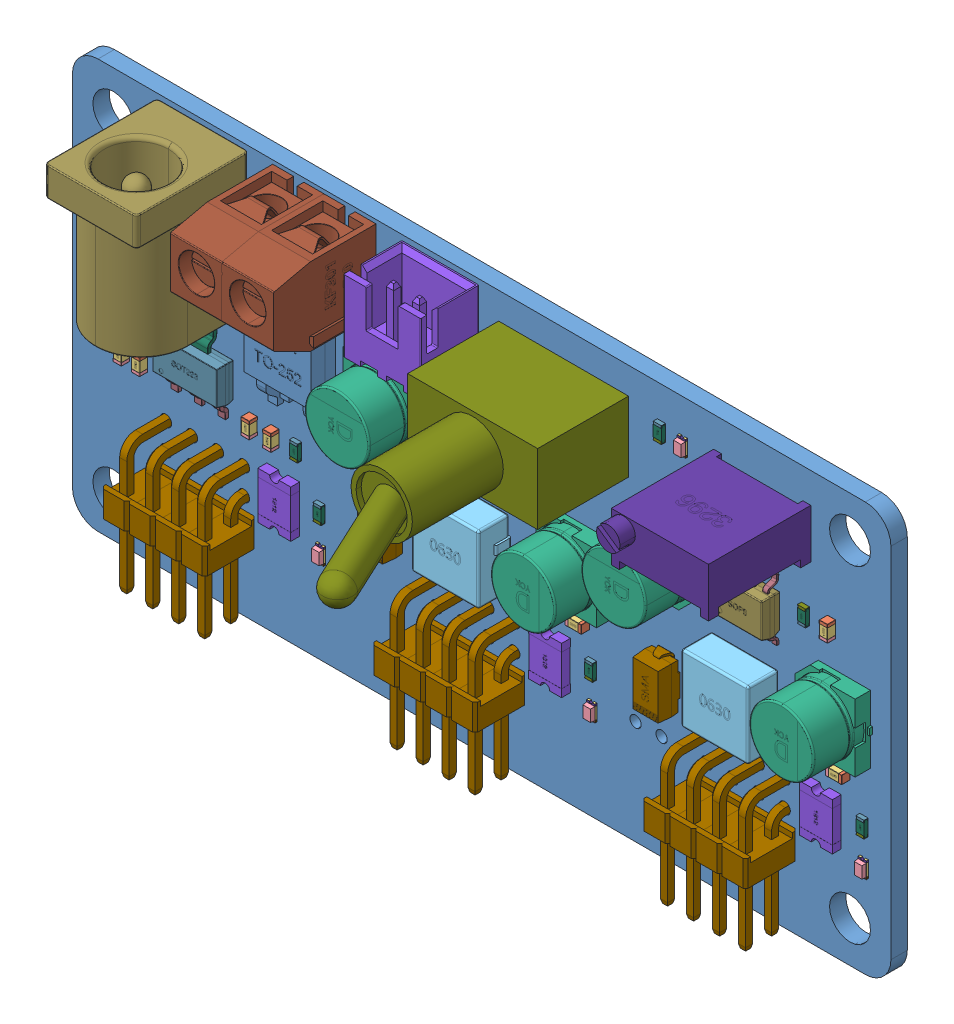
SolidWorks assembly PowerSupplyBoard, configuration 默认. Lengths in mm.
Overall size (80 40 32.5).
298 component instances, 37 part files, 0 mates.
Components (placement in the parent):
- PCB2.step-1: PCB2.step [默认] at origin size (80 40 32.5)
  - Board.step-1: Board.step [默认] at origin size (80 40 1.6)
    - Open CASCADE STEP translator 6.8 2.1.1.step-1: Open CASCADE STEP translator 6.8 2.1.1.step [默认] at (0 0 -1.6) size (80 40 1.6)
  - C1.step-1: C1.step [默认] at origin size (0.82 1.6 0.82)
    - C_0603.step-1: C_0603.step [默认] at (74.2189 27.7979 0.0254) x (0 -1 0) z (0 0 1) size (1.6 0.82 0.82)
      - C_0603-7177_AF0_ASM.step-1: C_0603-7177_AF0_ASM.step [默认] at origin size (1.6 0.82 0.82)
        - C_0603-683_AF0_ASM.step-1: C_0603-683_AF0_ASM.step [默认] at origin size (1.6 0.82 0.82)
          - 2_1_200.step-1: 2_1_200.step [默认] at origin size (0.3 0.82 0.82)
          - _1_1_20001.step-1: _1_1_20001.step [默认] at origin size (1 0.8 0.8)
          - 3_1_2_A.step-1: 3_1_2_A.step [默认] at origin size (0.3 0.82 0.82)
  - C3.step-1: C3.step [默认] at origin size (7 6.6 5.41)
    - CM_D(6.3X5.4).step-1: CM_D(6.3X5.4).step [默认] at (74.7014 21.0058 0) x (0 1 0) z (0 0 1) size (6.6 7 5.41)
      - LOGO_.step-1: LOGO_.step [默认] at (1.6383 0.2015 -0.0035) x (-1 0 0) z (0 0 -1) size (1.35 1.56 0.01)
      - CM_D(6.3X5.4)-0.step-1: CM_D(6.3X5.4)-0.step [默认] at origin size (6.6 7 5.41)
  - Open CASCADE STEP translator 6.8 2.4.step-1: Open CASCADE STEP translator 6.8 2.4.step [默认] at origin size (7.54 7.7 9.1)
    - XH2.54-2P_H.step-1: XH2.54-2P_H.step [默认] at (37.2618 32.1564 0.03) x (-1 0 0) z (0 1 0) size (7.54 9.1 7.7)
      - LOGO_-1.step-1: LOGO_-1.step [默认] at (-1.159 -0.003 2.4494) x (0 0 1) z (0 -1 0) size (0.9 1.04 0.01)
      - XH2.54-2P_H-2.step-1: XH2.54-2P_H-2.step [默认] at origin size (7.54 9.1 7.7)
  - Open CASCADE STEP translator 6.8 2.5.step-1: Open CASCADE STEP translator 6.8 2.5.step [默认] at origin size (10.16 12.85 8.1)
    - HDR-1x2_H.step-1: HDR-1x2_H.step [默认] at (40.6527 12.7 0) x (1 0 0) z (0 0 1) size (2.54 12.85 8.1)
      - HDR-1x2_H-3.step-1: HDR-1x2_H-3.step [默认] at origin size (2.54 12.85 8.1)
      - LOGO_-4.step-1: LOGO_-4.step [默认] at (0 -4.7829 0.017) x (-1 0 0) z (0 0 -1) size (0.9 1.04 0.01)
    - HDR-1x2_H.step-2: HDR-1x2_H.step [默认] at (43.1927 12.7 0) x (1 0 0) z (0 0 1) size (2.54 12.85 8.1)
      - HDR-1x2_H-3.step-1: HDR-1x2_H-3.step [默认] at origin size (2.54 12.85 8.1)
      - LOGO_-4.step-1: LOGO_-4.step [默认] at (0 -4.7829 0.017) x (-1 0 0) z (0 0 -1) size (0.9 1.04 0.01)
    - HDR-1x2_H.step-3: HDR-1x2_H.step [默认] at (35.5727 12.7 0) x (1 0 0) z (0 0 1) size (2.54 12.85 8.1)
      - HDR-1x2_H-3.step-1: HDR-1x2_H-3.step [默认] at origin size (2.54 12.85 8.1)
      - LOGO_-4.step-1: LOGO_-4.step [默认] at (0 -4.7829 0.017) x (-1 0 0) z (0 0 -1) size (0.9 1.04 0.01)
    - HDR-1x2_H.step-4: HDR-1x2_H.step [默认] at (38.1127 12.7 0) x (1 0 0) z (0 0 1) size (2.54 12.85 8.1)
      - HDR-1x2_H-3.step-1: HDR-1x2_H-3.step [默认] at origin size (2.54 12.85 8.1)
      - LOGO_-4.step-1: LOGO_-4.step [默认] at (0 -4.7829 0.017) x (-1 0 0) z (0 0 -1) size (0.9 1.04 0.01)
  - Open CASCADE STEP translator 6.8 2.6.step-1: Open CASCADE STEP translator 6.8 2.6.step [默认] at origin size (5 6.01 1.9)
    - SOP8.step-1: SOP8.step [默认] at (39.878 26.6954 0) x (0 1 0) z (0 0 1) size (6.01 5 1.9)
      - LOGO_0.25.step-1: LOGO_0.25.step [默认] at (0.0116 0 0.095) x (0 -1 0) z (0 0 -1) size (0.75 0.87 0.01)
      - SOP8_____.step-1: SOP8_____.step [默认] at origin size (3.6 5 1.8)
      - ____1.8_______.step-1: ____1.8_______.step [默认] at (1.8 1.91 1) x (0 1 0) z (0 0 1) size (0.5 1.2 1.1)
      - ____1.8_______.step-2: ____1.8_______.step [默认] at (1.8 0.64 1) x (0 1 0) z (0 0 1) size (0.5 1.2 1.1)
      - ____1.8_______.step-3: ____1.8_______.step [默认] at (1.8 -0.63 1) x (0 1 0) z (0 0 1) size (0.5 1.2 1.1)
      - ____1.8_______.step-4: ____1.8_______.step [默认] at (1.8 -1.9 1) x (0 1 0) z (0 0 1) size (0.5 1.2 1.1)
      - ____1.8_______.step-5: ____1.8_______.step [默认] at (-1.8 1.91 1) x (0 -1 0) z (0 0 1) size (0.5 1.2 1.1)
      - ____1.8_______.step-6: ____1.8_______.step [默认] at (-1.8 0.64 1) x (0 -1 0) z (0 0 1) size (0.5 1.2 1.1)
      - ____1.8_______.step-7: ____1.8_______.step [默认] at (-1.8 -0.63 1) x (0 -1 0) z (0 0 1) size (0.5 1.2 1.1)
      - ____1.8_______.step-8: ____1.8_______.step [默认] at (-1.8 -1.9 1) x (0 -1 0) z (0 0 1) size (0.5 1.2 1.1)
  - Open CASCADE STEP translator 6.8 2.7.step-1: Open CASCADE STEP translator 6.8 2.7.step [默认] at origin size (5 6.01 1.9)
    - SOP8.step-1: SOP8.step [默认] at (66.9036 26.6954 0) x (0 1 0) z (0 0 1) size (6.01 5 1.9)
      - LOGO_0.25.step-1: LOGO_0.25.step [默认] at (0.0116 0 0.095) x (0 -1 0) z (0 0 -1) size (0.75 0.87 0.01)
      - SOP8_____.step-1: SOP8_____.step [默认] at origin size (3.6 5 1.8)
      - ____1.8_______.step-1: ____1.8_______.step [默认] at (1.8 1.91 1) x (0 1 0) z (0 0 1) size (0.5 1.2 1.1)
      - ____1.8_______.step-2: ____1.8_______.step [默认] at (1.8 0.64 1) x (0 1 0) z (0 0 1) size (0.5 1.2 1.1)
      - ____1.8_______.step-3: ____1.8_______.step [默认] at (1.8 -0.63 1) x (0 1 0) z (0 0 1) size (0.5 1.2 1.1)
      - ____1.8_______.step-4: ____1.8_______.step [默认] at (1.8 -1.9 1) x (0 1 0) z (0 0 1) size (0.5 1.2 1.1)
      - ____1.8_______.step-5: ____1.8_______.step [默认] at (-1.8 1.91 1) x (0 -1 0) z (0 0 1) size (0.5 1.2 1.1)
      - ____1.8_______.step-6: ____1.8_______.step [默认] at (-1.8 0.64 1) x (0 -1 0) z (0 0 1) size (0.5 1.2 1.1)
      - ____1.8_______.step-7: ____1.8_______.step [默认] at (-1.8 -0.63 1) x (0 -1 0) z (0 0 1) size (0.5 1.2 1.1)
      - ____1.8_______.step-8: ____1.8_______.step [默认] at (-1.8 -1.9 1) x (0 -1 0) z (0 0 1) size (0.5 1.2 1.1)
  - R6.step-1: R6.step [默认] at origin size (0.8 1.6 0.4)
    - R0603.step-1: R0603.step [默认] at (44.6277 27.5996 0) x (0 1 0) z (0 0 1) size (1.6 0.8 0.4)
      - R_0603-3615_AF0_ASM.step-1: R_0603-3615_AF0_ASM.step [默认] at origin size (1.6 0.8 0.4)
        - R_0603-3601_AF0_ASM.step-1: R_0603-3601_AF0_ASM.step [默认] at origin size (1.6 0.8 0.4)
          - _2_1_2_3_4_AF0.step-1: _2_1_2_3_4_AF0.step [默认] at origin size (0.25 0.8 0.4)
          - _7_1_2_AF0.step-1: _7_1_2_AF0.step [默认] at origin size (1.5 0.8 0.4)
          - 5_1_2_3_400.step-1: 5_1_2_3_400.step [默认] at origin size (0.25 0.8 0.4)
  - R5.step-1: R5.step [默认] at origin size (0.8 1.6 0.4)
    - R0603.step-1: R0603.step [默认] at (50.8338 12.5832 0) x (0 -1 0) z (0 0 1) size (1.6 0.8 0.4)
      - R_0603-3615_AF0_ASM.step-1: R_0603-3615_AF0_ASM.step [默认] at origin size (1.6 0.8 0.4)
        - R_0603-3601_AF0_ASM.step-1: R_0603-3601_AF0_ASM.step [默认] at origin size (1.6 0.8 0.4)
          - _2_1_2_3_4_AF0.step-1: _2_1_2_3_4_AF0.step [默认] at origin size (0.25 0.8 0.4)
          - _7_1_2_AF0.step-1: _7_1_2_AF0.step [默认] at origin size (1.5 0.8 0.4)
          - 5_1_2_3_400.step-1: 5_1_2_3_400.step [默认] at origin size (0.25 0.8 0.4)
  - R4.step-1: R4.step [默认] at origin size (0.8 1.6 0.4)
    - R0603.step-1: R0603.step [默认] at (47.2185 27.5996 0) x (0 1 0) z (0 0 1) size (1.6 0.8 0.4)
      - R_0603-3615_AF0_ASM.step-1: R_0603-3615_AF0_ASM.step [默认] at origin size (1.6 0.8 0.4)
        - R_0603-3601_AF0_ASM.step-1: R_0603-3601_AF0_ASM.step [默认] at origin size (1.6 0.8 0.4)
          - _2_1_2_3_4_AF0.step-1: _2_1_2_3_4_AF0.step [默认] at origin size (0.25 0.8 0.4)
          - _7_1_2_AF0.step-1: _7_1_2_AF0.step [默认] at origin size (1.5 0.8 0.4)
          - 5_1_2_3_400.step-1: 5_1_2_3_400.step [默认] at origin size (0.25 0.8 0.4)
  - LED2.step-1: LED2.step [默认] at origin size (0.8 1.6 0.61)
    - LED_0603-G(1).step-1: LED_0603-G(1).step [默认] at (50.8649 9.0649 0) x (0 1 0) z (0 0 1) size (1.6 0.8 0.47)
      - LED_0603-G-7058_AF0_ASM.step-1: LED_0603-G-7058_AF0_ASM.step [默认] at origin size (1.6 0.8 0.47)
        - LED_0603-G-4339_AF0_ASM.step-1: LED_0603-G-4339_AF0_ASM.step [默认] at origin size (1.6 0.8 0.47)
          - 4_100.step-1: 4_100.step [默认] at origin size (0.2 0.8 0.2)
          - _2_10001.step-1: _2_10001.step [默认] at origin size (0.2 0.8 0.2)
          - _5_2__10001.step-1: _5_2__10001.step [默认] at origin size (0.31 0.14 0)
          - _5_1__10001.step-1: _5_1__10001.step [默认] at origin size (0.31 0.14 0)
          - 1_1_2_3_4_5_6_7_8_0.step-1: 1_1_2_3_4_5_6_7_8_0.step [默认] at origin size (1.6 0.8 0.47)
    - LED_0603______.step-1: LED_0603______.step [默认] at (50.8649 9.0649 0) x (0 -1 0) z (0 0 1) size (1.2 0.8 0.4)
  - Open CASCADE STEP translator 6.8 2.12.step-1: Open CASCADE STEP translator 6.8 2.12.step [默认] at origin size (6.95 6.6 3.03)
    - SMD-0630.step-1: SMD-0630.step [默认] at (39.4682 18.3134 0) x (1 0 0) z (0 0 1) size (6.95 6.6 3.03)
      - SMD-0630-5.step-1: SMD-0630-5.step [默认] at origin size (6.95 6.6 3.03)
      - LOGO_0.5.step-1: LOGO_0.5.step [默认] at (0 0.0017 0.04) size (1.5 1.73 0.01)
  - F2.step-1: F2.step [默认] at origin size (3.22 4.6 0.87)
    - FU_01812.step-1: FU_01812.step [默认] at (47.0662 11.7496 0) x (0 -1 0) z (0 0 1) size (4.6 3.22 0.87)
      - LOGO_-6.step-1: LOGO_-6.step [默认] at (0 0.0363 0.009) x (-1 0 0) z (0 0 -1) size (0.6 0.69 0)
      - FU_1812.step-1: FU_1812.step [默认] at origin size (4.6 3.22 0.87)
  - D2.step-1: D2.step [默认] at origin size (2.6 5.12 2.1)
    - SMA.step-1: SMA.step [默认] at (31.2327 15.471 0.0508) x (0 1 0) z (0 0 1) size (5.12 2.6 2.1)
      - SMA-4715_AF0_ASM.step-1: SMA-4715_AF0_ASM.step [默认] at origin size (5.12 2.6 2.1)
        - SMA-5401_AF0.step-1: SMA-5401_AF0.step [默认] at origin size (5.12 2.6 2.1)
  - C12.step-1: C12.step [默认] at origin size (0.82 1.6 0.82)
    - C_0603.step-1: C_0603.step [默认] at (6.9851 16.7489 0.0254) x (0 -1 0) z (0 0 1) size (1.6 0.82 0.82)
      - C_0603-7177_AF0_ASM.step-1: C_0603-7177_AF0_ASM.step [默认] at origin size (1.6 0.82 0.82)
        - C_0603-683_AF0_ASM.step-1: C_0603-683_AF0_ASM.step [默认] at origin size (1.6 0.82 0.82)
          - 2_1_200.step-1: 2_1_200.step [默认] at origin size (0.3 0.82 0.82)
          - _1_1_20001.step-1: _1_1_20001.step [默认] at origin size (1 0.8 0.8)
          - 3_1_2_A.step-1: 3_1_2_A.step [默认] at origin size (0.3 0.82 0.82)
  - C10.step-1: C10.step [默认] at origin size (0.82 1.6 0.82)
    - C_0603.step-1: C_0603.step [默认] at (19.8248 16.7489 0.0254) x (0 -1 0) z (0 0 1) size (1.6 0.82 0.82)
      - C_0603-7177_AF0_ASM.step-1: C_0603-7177_AF0_ASM.step [默认] at origin size (1.6 0.82 0.82)
        - C_0603-683_AF0_ASM.step-1: C_0603-683_AF0_ASM.step [默认] at origin size (1.6 0.82 0.82)
          - 2_1_200.step-1: 2_1_200.step [默认] at origin size (0.3 0.82 0.82)
          - _1_1_20001.step-1: _1_1_20001.step [默认] at origin size (1 0.8 0.8)
          - 3_1_2_A.step-1: 3_1_2_A.step [默认] at origin size (0.3 0.82 0.82)
  - C9.step-1: C9.step [默认] at origin size (1.6 0.82 0.82)
    - C_0603.step-1: C_0603.step [默认] at (49.7689 16.1289 0.0254) x (-1 0 0) z (0 0 1) size (1.6 0.82 0.82)
      - C_0603-7177_AF0_ASM.step-1: C_0603-7177_AF0_ASM.step [默认] at origin size (1.6 0.82 0.82)
        - C_0603-683_AF0_ASM.step-1: C_0603-683_AF0_ASM.step [默认] at origin size (1.6 0.82 0.82)
          - 2_1_200.step-1: 2_1_200.step [默认] at origin size (0.3 0.82 0.82)
          - _1_1_20001.step-1: _1_1_20001.step [默认] at origin size (1 0.8 0.8)
          - 3_1_2_A.step-1: 3_1_2_A.step [默认] at origin size (0.3 0.82 0.82)
  - C8.step-1: C8.step [默认] at origin size (0.82 1.6 0.82)
    - C_0603.step-1: C_0603.step [默认] at (35.9681 25.8961 0.0254) x (0 -1 0) z (0 0 1) size (1.6 0.82 0.82)
      - C_0603-7177_AF0_ASM.step-1: C_0603-7177_AF0_ASM.step [默认] at origin size (1.6 0.82 0.82)
        - C_0603-683_AF0_ASM.step-1: C_0603-683_AF0_ASM.step [默认] at origin size (1.6 0.82 0.82)
          - 2_1_200.step-1: 2_1_200.step [默认] at origin size (0.3 0.82 0.82)
          - _1_1_20001.step-1: _1_1_20001.step [默认] at origin size (1 0.8 0.8)
          - 3_1_2_A.step-1: 3_1_2_A.step [默认] at origin size (0.3 0.82 0.82)
  - C7.step-1: C7.step [默认] at origin size (7 6.6 5.41)
    - CM_D(6.3X5.4).step-1: CM_D(6.3X5.4).step [默认] at (49.4284 21.0058 0) x (0 1 0) z (0 0 1) size (6.6 7 5.41)
      - LOGO_.step-1: LOGO_.step [默认] at (1.6383 0.2015 -0.0035) x (-1 0 0) z (0 0 -1) size (1.35 1.56 0.01)
      - CM_D(6.3X5.4)-0.step-1: CM_D(6.3X5.4)-0.step [默认] at origin size (6.6 7 5.41)
  - C6.step-1: C6.step [默认] at origin size (6.6 7 5.41)
    - CM_D(6.3X5.4).step-1: CM_D(6.3X5.4).step [默认] at (31.242 25.8318 0) x (-1 0 0) z (0 0 1) size (6.6 7 5.41)
      - LOGO_.step-1: LOGO_.step [默认] at (1.6383 0.2015 -0.0035) x (-1 0 0) z (0 0 -1) size (1.35 1.56 0.01)
      - CM_D(6.3X5.4)-0.step-1: CM_D(6.3X5.4)-0.step [默认] at origin size (6.6 7 5.41)
  - C13.step-1: C13.step [默认] at origin size (0.82 1.6 0.82)
    - C_0603.step-1: C_0603.step [默认] at (5.2071 16.7489 0.0254) x (0 -1 0) z (0 0 1) size (1.6 0.82 0.82)
      - C_0603-7177_AF0_ASM.step-1: C_0603-7177_AF0_ASM.step [默认] at origin size (1.6 0.82 0.82)
        - C_0603-683_AF0_ASM.step-1: C_0603-683_AF0_ASM.step [默认] at origin size (1.6 0.82 0.82)
          - 2_1_200.step-1: 2_1_200.step [默认] at origin size (0.3 0.82 0.82)
          - _1_1_20001.step-1: _1_1_20001.step [默认] at origin size (1 0.8 0.8)
          - 3_1_2_A.step-1: 3_1_2_A.step [默认] at origin size (0.3 0.82 0.82)
  - Open CASCADE STEP translator 6.8 2.22.step-1: Open CASCADE STEP translator 6.8 2.22.step [默认] at origin size (10.5 7.6 13.8)
    - KF301.step-1: KF301.step [默认] at (27.1742 36.6776 0.05) x (-1 0 0) z (0 0 1) size (5.5 7.6 13.8)
      - LOGO_-7.step-1: LOGO_-7.step [默认] at (0 1.4435 -0.0028) x (-1 0 0) z (0 0 -1) size (0.84 0.97 0.01)
      - KF301-8.step-1: KF301-8.step [默认] x (1 0 0) z (0 -1 0) size (5.5 13.8 7.6)
    - KF301.step-2: KF301.step [默认] at (22.1742 36.6776 0.05) x (-1 0 0) z (0 0 1) size (5.5 7.6 13.8)
      - LOGO_-7.step-1: LOGO_-7.step [默认] at (0 1.4435 -0.0028) x (-1 0 0) z (0 0 -1) size (0.84 0.97 0.01)
      - KF301-8.step-1: KF301-8.step [默认] x (1 0 0) z (0 -1 0) size (5.5 13.8 7.6)
  - Open CASCADE STEP translator 6.8 2.23.step-1: Open CASCADE STEP translator 6.8 2.23.step [默认] at origin size (9.3 14.05 15)
    - dc-005.step-1: dc-005.step [默认] at (12.9532 32.2582 0.2) x (-1 0 0) z (0 0 1) size (9.3 14.05 15)
  - C5.step-1: C5.step [默认] at origin size (1.6 0.82 0.82)
    - C_0603.step-1: C_0603.step [默认] at (75.2197 16.1289 0.0254) x (-1 0 0) z (0 0 1) size (1.6 0.82 0.82)
      - C_0603-7177_AF0_ASM.step-1: C_0603-7177_AF0_ASM.step [默认] at origin size (1.6 0.82 0.82)
        - C_0603-683_AF0_ASM.step-1: C_0603-683_AF0_ASM.step [默认] at origin size (1.6 0.82 0.82)
          - 2_1_200.step-1: 2_1_200.step [默认] at origin size (0.3 0.82 0.82)
          - _1_1_20001.step-1: _1_1_20001.step [默认] at origin size (1 0.8 0.8)
          - 3_1_2_A.step-1: 3_1_2_A.step [默认] at origin size (0.3 0.82 0.82)
  - Open CASCADE STEP translator 6.8 2.25.step-1: Open CASCADE STEP translator 6.8 2.25.step [默认] at origin size (6.51 7.02 1.67)
    - SOT223.step-1: SOT223.step [默认] at (12.6231 19.5037 0) x (1 0 0) z (0 0 1) size (6.51 7.02 1.67)
      - SOT223-4091_AF0_ASM.step-1: SOT223-4091_AF0_ASM.step [默认] at origin size (6.51 7.02 1.67)
        - SOT223_-20.step-1: SOT223_-20.step [默认] at (-2.3 -1.75 0.725) x (-1 0 0) z (0 0 1) size (0.71 1.76 0.92)
        - SOT223-16115_AF0.step-1: SOT223-16115_AF0.step [默认] at origin size (6.51 3.51 1.6)
        - SOT223_-10.step-1: SOT223_-10.step [默认] at (0 1.75 0.725) size (3 1.76 0.92)
        - SOT223_-20.step-2: SOT223_-20.step [默认] at (2.3 -1.75 0.725) x (-1 0 0) z (0 0 1) size (0.71 1.76 0.92)
        - SOT223_-20.step-3: SOT223_-20.step [默认] at (0 -1.75 0.725) x (-1 0 0) z (0 0 1) size (0.71 1.76 0.92)
  - S1.step-1: S1.step [默认] at origin size (12.72 10.16 32.39)
    - User_Library-7101SYZQE_switch-toggle.step-1: User_Library-7101SYZQE_switch-toggle.step [默认] at (48.26 34.2138 9.144) x (0 0 -1) z (1 0 0) size (32.39 10.16 12.72)
  - R9.step-1: R9.step [默认] at origin size (0.8 1.6 0.4)
    - R0603.step-1: R0603.step [默认] at (57.5666 36.0794 0) x (0 -1 0) z (0 0 1) size (1.6 0.8 0.4)
      - R_0603-3615_AF0_ASM.step-1: R_0603-3615_AF0_ASM.step [默认] at origin size (1.6 0.8 0.4)
        - R_0603-3601_AF0_ASM.step-1: R_0603-3601_AF0_ASM.step [默认] at origin size (1.6 0.8 0.4)
          - _2_1_2_3_4_AF0.step-1: _2_1_2_3_4_AF0.step [默认] at origin size (0.25 0.8 0.4)
          - _7_1_2_AF0.step-1: _7_1_2_AF0.step [默认] at origin size (1.5 0.8 0.4)
          - 5_1_2_3_400.step-1: 5_1_2_3_400.step [默认] at origin size (0.25 0.8 0.4)
  - R8.step-1: R8.step [默认] at origin size (0.8 1.6 0.4)
    - R0603.step-1: R0603.step [默认] at (21.9965 16.7234 0) x (0 -1 0) z (0 0 1) size (1.6 0.8 0.4)
      - R_0603-3615_AF0_ASM.step-1: R_0603-3615_AF0_ASM.step [默认] at origin size (1.6 0.8 0.4)
        - R_0603-3601_AF0_ASM.step-1: R_0603-3601_AF0_ASM.step [默认] at origin size (1.6 0.8 0.4)
          - _2_1_2_3_4_AF0.step-1: _2_1_2_3_4_AF0.step [默认] at origin size (0.25 0.8 0.4)
          - _7_1_2_AF0.step-1: _7_1_2_AF0.step [默认] at origin size (1.5 0.8 0.4)
          - 5_1_2_3_400.step-1: 5_1_2_3_400.step [默认] at origin size (0.25 0.8 0.4)
  - R7.step-1: R7.step [默认] at origin size (0.8 1.6 0.4)
    - R0603.step-1: R0603.step [默认] at (24.2991 12.5832 0) x (0 -1 0) z (0 0 1) size (1.6 0.8 0.4)
      - R_0603-3615_AF0_ASM.step-1: R_0603-3615_AF0_ASM.step [默认] at origin size (1.6 0.8 0.4)
        - R_0603-3601_AF0_ASM.step-1: R_0603-3601_AF0_ASM.step [默认] at origin size (1.6 0.8 0.4)
          - _2_1_2_3_4_AF0.step-1: _2_1_2_3_4_AF0.step [默认] at origin size (0.25 0.8 0.4)
          - _7_1_2_AF0.step-1: _7_1_2_AF0.step [默认] at origin size (1.5 0.8 0.4)
          - 5_1_2_3_400.step-1: 5_1_2_3_400.step [默认] at origin size (0.25 0.8 0.4)
  - R3.step-1: R3.step [默认] at origin size (0.8 1.6 0.4)
    - R0603.step-1: R0603.step [默认] at (77.3685 12.5832 0) x (0 -1 0) z (0 0 1) size (1.6 0.8 0.4)
      - R_0603-3615_AF0_ASM.step-1: R_0603-3615_AF0_ASM.step [默认] at origin size (1.6 0.8 0.4)
        - R_0603-3601_AF0_ASM.step-1: R_0603-3601_AF0_ASM.step [默认] at origin size (1.6 0.8 0.4)
          - _2_1_2_3_4_AF0.step-1: _2_1_2_3_4_AF0.step [默认] at origin size (0.25 0.8 0.4)
          - _7_1_2_AF0.step-1: _7_1_2_AF0.step [默认] at origin size (1.5 0.8 0.4)
          - 5_1_2_3_400.step-1: 5_1_2_3_400.step [默认] at origin size (0.25 0.8 0.4)
  - R2.step-1: R2.step [默认] at origin size (9.5 4.8 15)
    - 3296.step-1: 3296.step [默认] at (67.4409 34.6711 0.02) x (-1 0 0) z (0 0 1) size (9.5 4.8 15)
      - 3296-10.step-1: 3296-10.step [默认] at origin size (9.5 4.8 15)
      - LOGO_-11.step-1: LOGO_-11.step [默认] at (1.2121 -0.8676 0.494) x (-1 0 0) z (0 0 -1) size (1.8 2.08 0.01)
  - R1.step-1: R1.step [默认] at origin size (0.8 1.6 0.4)
    - R0603.step-1: R0603.step [默认] at (71.6533 27.5996 0) x (0 1 0) z (0 0 1) size (1.6 0.8 0.4)
      - R_0603-3615_AF0_ASM.step-1: R_0603-3615_AF0_ASM.step [默认] at origin size (1.6 0.8 0.4)
        - R_0603-3601_AF0_ASM.step-1: R_0603-3601_AF0_ASM.step [默认] at origin size (1.6 0.8 0.4)
          - _2_1_2_3_4_AF0.step-1: _2_1_2_3_4_AF0.step [默认] at origin size (0.25 0.8 0.4)
          - _7_1_2_AF0.step-1: _7_1_2_AF0.step [默认] at origin size (1.5 0.8 0.4)
          - 5_1_2_3_400.step-1: 5_1_2_3_400.step [默认] at origin size (0.25 0.8 0.4)
  - Q1.step-1: Q1.step [默认] at origin size (6.73 10.1 2.4)
    - DPAK_TO-252AA.step-1: DPAK_TO-252AA.step [默认] at (22.5553 26.1736 0.127) x (1 0 0) z (0 -1 0) size (6.73 2.4 10.1)
  - LED4.step-1: LED4.step [默认] at origin size (0.8 1.6 0.61)
    - LED_0603-G(1).step-1: LED_0603-G(1).step [默认] at (59.7183 35.8962 0) x (0 1 0) z (0 0 1) size (1.6 0.8 0.47)
      - LED_0603-G-7058_AF0_ASM.step-1: LED_0603-G-7058_AF0_ASM.step [默认] at origin size (1.6 0.8 0.47)
        - LED_0603-G-4339_AF0_ASM.step-1: LED_0603-G-4339_AF0_ASM.step [默认] at origin size (1.6 0.8 0.47)
          - 4_100.step-1: 4_100.step [默认] at origin size (0.2 0.8 0.2)
          - _2_10001.step-1: _2_10001.step [默认] at origin size (0.2 0.8 0.2)
          - _5_2__10001.step-1: _5_2__10001.step [默认] at origin size (0.31 0.14 0)
          - _5_1__10001.step-1: _5_1__10001.step [默认] at origin size (0.31 0.14 0)
          - 1_1_2_3_4_5_6_7_8_0.step-1: 1_1_2_3_4_5_6_7_8_0.step [默认] at origin size (1.6 0.8 0.47)
    - LED_0603______.step-1: LED_0603______.step [默认] at (59.7183 35.8962 0) x (0 -1 0) z (0 0 1) size (1.2 0.8 0.4)
  - LED3.step-1: LED3.step [默认] at origin size (0.8 1.6 0.61)
    - LED_0603-G(1).step-1: LED_0603-G(1).step [默认] at (24.3395 9.0649 0) x (0 1 0) z (0 0 1) size (1.6 0.8 0.47)
      - LED_0603-G-7058_AF0_ASM.step-1: LED_0603-G-7058_AF0_ASM.step [默认] at origin size (1.6 0.8 0.47)
        - LED_0603-G-4339_AF0_ASM.step-1: LED_0603-G-4339_AF0_ASM.step [默认] at origin size (1.6 0.8 0.47)
          - 4_100.step-1: 4_100.step [默认] at origin size (0.2 0.8 0.2)
          - _2_10001.step-1: _2_10001.step [默认] at origin size (0.2 0.8 0.2)
          - _5_2__10001.step-1: _5_2__10001.step [默认] at origin size (0.31 0.14 0)
          - _5_1__10001.step-1: _5_1__10001.step [默认] at origin size (0.31 0.14 0)
          - 1_1_2_3_4_5_6_7_8_0.step-1: 1_1_2_3_4_5_6_7_8_0.step [默认] at origin size (1.6 0.8 0.47)
    - LED_0603______.step-1: LED_0603______.step [默认] at (24.3395 9.0649 0) x (0 -1 0) z (0 0 1) size (1.2 0.8 0.4)
  - LED1.step-1: LED1.step [默认] at origin size (0.8 1.6 0.61)
    - LED_0603-G(1).step-1: LED_0603-G(1).step [默认] at (77.3902 9.0649 0) x (0 1 0) z (0 0 1) size (1.6 0.8 0.47)
      - LED_0603-G-7058_AF0_ASM.step-1: LED_0603-G-7058_AF0_ASM.step [默认] at origin size (1.6 0.8 0.47)
        - LED_0603-G-4339_AF0_ASM.step-1: LED_0603-G-4339_AF0_ASM.step [默认] at origin size (1.6 0.8 0.47)
          - 4_100.step-1: 4_100.step [默认] at origin size (0.2 0.8 0.2)
          - _2_10001.step-1: _2_10001.step [默认] at origin size (0.2 0.8 0.2)
          - _5_2__10001.step-1: _5_2__10001.step [默认] at origin size (0.31 0.14 0)
          - _5_1__10001.step-1: _5_1__10001.step [默认] at origin size (0.31 0.14 0)
          - 1_1_2_3_4_5_6_7_8_0.step-1: 1_1_2_3_4_5_6_7_8_0.step [默认] at origin size (1.6 0.8 0.47)
    - LED_0603______.step-1: LED_0603______.step [默认] at (77.3902 9.0649 0) x (0 -1 0) z (0 0 1) size (1.2 0.8 0.4)
  - Open CASCADE STEP translator 6.8 2.37.step-1: Open CASCADE STEP translator 6.8 2.37.step [默认] at origin size (6.95 6.6 3.03)
    - SMD-0630.step-1: SMD-0630.step [默认] at (65.808 18.3134 0) x (1 0 0) z (0 0 1) size (6.95 6.6 3.03)
      - SMD-0630-5.step-1: SMD-0630-5.step [默认] at origin size (6.95 6.6 3.03)
      - LOGO_0.5.step-1: LOGO_0.5.step [默认] at (0 0.0017 0.04) size (1.5 1.73 0.01)
  - Open CASCADE STEP translator 6.8 2.38.step-1: Open CASCADE STEP translator 6.8 2.38.step [默认] at origin size (10.16 12.85 8.1)
    - HDR-1x2_H.step-1: HDR-1x2_H.step [默认] at (14.224 12.7 0) x (1 0 0) z (0 0 1) size (2.54 12.85 8.1)
      - HDR-1x2_H-3.step-1: HDR-1x2_H-3.step [默认] at origin size (2.54 12.85 8.1)
      - LOGO_-4.step-1: LOGO_-4.step [默认] at (0 -4.7829 0.017) x (-1 0 0) z (0 0 -1) size (0.9 1.04 0.01)
    - HDR-1x2_H.step-2: HDR-1x2_H.step [默认] at (16.764 12.7 0) x (1 0 0) z (0 0 1) size (2.54 12.85 8.1)
      - HDR-1x2_H-3.step-1: HDR-1x2_H-3.step [默认] at origin size (2.54 12.85 8.1)
      - LOGO_-4.step-1: LOGO_-4.step [默认] at (0 -4.7829 0.017) x (-1 0 0) z (0 0 -1) size (0.9 1.04 0.01)
    - HDR-1x2_H.step-3: HDR-1x2_H.step [默认] at (9.144 12.7 0) x (1 0 0) z (0 0 1) size (2.54 12.85 8.1)
      - HDR-1x2_H-3.step-1: HDR-1x2_H-3.step [默认] at origin size (2.54 12.85 8.1)
      - LOGO_-4.step-1: LOGO_-4.step [默认] at (0 -4.7829 0.017) x (-1 0 0) z (0 0 -1) size (0.9 1.04 0.01)
    - HDR-1x2_H.step-4: HDR-1x2_H.step [默认] at (11.684 12.7 0) x (1 0 0) z (0 0 1) size (2.54 12.85 8.1)
      - HDR-1x2_H-3.step-1: HDR-1x2_H-3.step [默认] at origin size (2.54 12.85 8.1)
      - LOGO_-4.step-1: LOGO_-4.step [默认] at (0 -4.7829 0.017) x (-1 0 0) z (0 0 -1) size (0.9 1.04 0.01)
  - Open CASCADE STEP translator 6.8 2.39.step-1: Open CASCADE STEP translator 6.8 2.39.step [默认] at origin size (10.16 12.85 8.1)
    - HDR-1x2_H.step-1: HDR-1x2_H.step [默认] at (67.0814 12.7 0) x (1 0 0) z (0 0 1) size (2.54 12.85 8.1)
      - HDR-1x2_H-3.step-1: HDR-1x2_H-3.step [默认] at origin size (2.54 12.85 8.1)
      - LOGO_-4.step-1: LOGO_-4.step [默认] at (0 -4.7829 0.017) x (-1 0 0) z (0 0 -1) size (0.9 1.04 0.01)
    - HDR-1x2_H.step-2: HDR-1x2_H.step [默认] at (69.6214 12.7 0) x (1 0 0) z (0 0 1) size (2.54 12.85 8.1)
      - HDR-1x2_H-3.step-1: HDR-1x2_H-3.step [默认] at origin size (2.54 12.85 8.1)
      - LOGO_-4.step-1: LOGO_-4.step [默认] at (0 -4.7829 0.017) x (-1 0 0) z (0 0 -1) size (0.9 1.04 0.01)
    - HDR-1x2_H.step-3: HDR-1x2_H.step [默认] at (62.0014 12.7 0) x (1 0 0) z (0 0 1) size (2.54 12.85 8.1)
      - HDR-1x2_H-3.step-1: HDR-1x2_H-3.step [默认] at origin size (2.54 12.85 8.1)
      - LOGO_-4.step-1: LOGO_-4.step [默认] at (0 -4.7829 0.017) x (-1 0 0) z (0 0 -1) size (0.9 1.04 0.01)
    - HDR-1x2_H.step-4: HDR-1x2_H.step [默认] at (64.5414 12.7 0) x (1 0 0) z (0 0 1) size (2.54 12.85 8.1)
      - HDR-1x2_H-3.step-1: HDR-1x2_H-3.step [默认] at origin size (2.54 12.85 8.1)
      - LOGO_-4.step-1: LOGO_-4.step [默认] at (0 -4.7829 0.017) x (-1 0 0) z (0 0 -1) size (0.9 1.04 0.01)
  - F3.step-1: F3.step [默认] at origin size (3.22 4.6 0.87)
    - FU_01812.step-1: FU_01812.step [默认] at (20.5994 11.7496 0) x (0 -1 0) z (0 0 1) size (4.6 3.22 0.87)
      - LOGO_-6.step-1: LOGO_-6.step [默认] at (0 0.0363 0.009) x (-1 0 0) z (0 0 -1) size (0.6 0.69 0)
      - FU_1812.step-1: FU_1812.step [默认] at origin size (4.6 3.22 0.87)
  - F1.step-1: F1.step [默认] at origin size (3.22 4.6 0.87)
    - FU_01812.step-1: FU_01812.step [默认] at (73.533 11.7496 0) x (0 -1 0) z (0 0 1) size (4.6 3.22 0.87)
      - LOGO_-6.step-1: LOGO_-6.step [默认] at (0 0.0363 0.009) x (-1 0 0) z (0 0 -1) size (0.6 0.69 0)
      - FU_1812.step-1: FU_1812.step [默认] at origin size (4.6 3.22 0.87)
  - D1.step-1: D1.step [默认] at origin size (2.6 5.12 2.1)
    - SMA.step-1: SMA.step [默认] at (58.1567 15.471 0.0508) x (0 1 0) z (0 0 1) size (5.12 2.6 2.1)
      - SMA-4715_AF0_ASM.step-1: SMA-4715_AF0_ASM.step [默认] at origin size (5.12 2.6 2.1)
        - SMA-5401_AF0.step-1: SMA-5401_AF0.step [默认] at origin size (5.12 2.6 2.1)
  - C11.step-1: C11.step [默认] at origin size (0.82 1.6 0.82)
    - C_0603.step-1: C_0603.step [默认] at (17.7039 16.7489 0.0254) x (0 -1 0) z (0 0 1) size (1.6 0.82 0.82)
      - C_0603-7177_AF0_ASM.step-1: C_0603-7177_AF0_ASM.step [默认] at origin size (1.6 0.82 0.82)
        - C_0603-683_AF0_ASM.step-1: C_0603-683_AF0_ASM.step [默认] at origin size (1.6 0.82 0.82)
          - 2_1_200.step-1: 2_1_200.step [默认] at origin size (0.3 0.82 0.82)
          - _1_1_20001.step-1: _1_1_20001.step [默认] at origin size (1 0.8 0.8)
          - 3_1_2_A.step-1: 3_1_2_A.step [默认] at origin size (0.3 0.82 0.82)
  - C4.step-1: C4.step [默认] at origin size (0.82 1.6 0.82)
    - C_0603.step-1: C_0603.step [默认] at (63.0175 25.8961 0.0254) x (0 -1 0) z (0 0 1) size (1.6 0.82 0.82)
      - C_0603-7177_AF0_ASM.step-1: C_0603-7177_AF0_ASM.step [默认] at origin size (1.6 0.82 0.82)
        - C_0603-683_AF0_ASM.step-1: C_0603-683_AF0_ASM.step [默认] at origin size (1.6 0.82 0.82)
          - 2_1_200.step-1: 2_1_200.step [默认] at origin size (0.3 0.82 0.82)
          - _1_1_20001.step-1: _1_1_20001.step [默认] at origin size (1 0.8 0.8)
          - 3_1_2_A.step-1: 3_1_2_A.step [默认] at origin size (0.3 0.82 0.82)
  - C2.step-1: C2.step [默认] at origin size (6.6 7 5.41)
    - CM_D(6.3X5.4).step-1: CM_D(6.3X5.4).step [默认] at (58.2676 25.8318 0) x (-1 0 0) z (0 0 1) size (6.6 7 5.41)
      - LOGO_.step-1: LOGO_.step [默认] at (1.6383 0.2015 -0.0035) x (-1 0 0) z (0 0 -1) size (1.35 1.56 0.01)
      - CM_D(6.3X5.4)-0.step-1: CM_D(6.3X5.4)-0.step [默认] at origin size (6.6 7 5.41)
